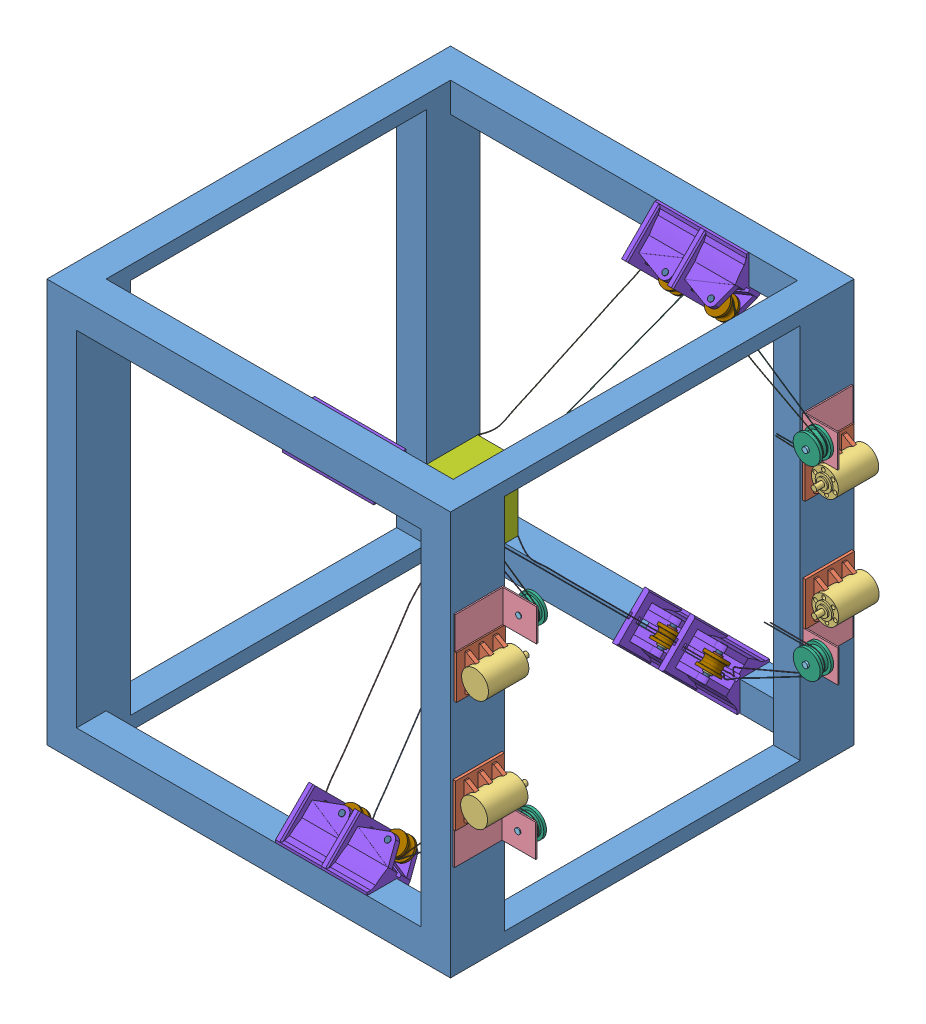
SolidWorks assembly 四自由度悬索机器人-粗装3, configuration 默认. Lengths in mm.
Overall size (1630.53 1500 1500).
86 component instances, 20 part files, 27 mates.
Components (placement in the parent):
- 框架-1: 框架 [默认] at (-869.4424 -713.1507 2250) size (1500 1500 1500)
- 驱动器-装配1-1: 驱动器-装配1 [默认] at (664.6049 -149.4407 667.2739) x (0 -1 0) z (0 0 1) size (280.09 130 239.56)
  - 驱动器--电机底座-1: 驱动器--电机底座 [默认] at (10.8985 -19.0474 121.978) size (160.09 50.28 181.98)
  - 驱动器-电机-1: 驱动器-电机 [默认] at (10.8985 30.9526 104.6663) x (0.931838 -0.362873 0) z (0 0 1) size (100 100 191)
  - 驱动器-滑轮组基座-1: 驱动器-滑轮组基座 [默认] at (90.9444 -34.0474 272.849) size (120 130 181.86)
  - 驱动器-定滑轮轴-1: 驱动器-定滑轮轴 [默认] at (150.9444 30.9526 265.5462) x (0.990128 -0.140168 0) z (0 0 1) size (20 20 65)
  - 驱动器-定滑轮-1: 驱动器-定滑轮 [默认] at (150.9167 30.9894 273.7821) x (0.990128 -0.140168 0) z (0 0 1) size (100 100 50)
- 驱动器-装配2-1: 驱动器-装配2 [默认] at (664.6049 262.8868 668.7376) x (0 -1 0) z (0 0 1) size (280.77 130.53 238.87)
  - 驱动器--电机底座-1: 驱动器--电机底座 [默认] at (10.8985 -19.0474 121.978) size (160.09 50.28 181.98)
  - 驱动器-电机-1: 驱动器-电机 [默认] at (10.8985 30.9526 104.6663) x (0.931838 -0.362873 0) z (0 0 1) size (100 100 191)
  - 驱动器-滑轮组基座-1: 驱动器-滑轮组基座 [默认] at (-189.8227 -33.5134 273.0905) size (120 130 181.86)
  - 驱动器-定滑轮轴-1: 驱动器-定滑轮轴 [默认] at (-129.7901 31.454 264.8545) size (20 20 65)
  - 驱动器-定滑轮-1: 驱动器-定滑轮 [默认] at (-129.8227 31.4866 273.0905) size (100 100 50)
- 驱动器-装配3-1: 驱动器-装配3 [默认] at (664.6049 -169.9542 2331.8379) x (0 1 0) z (0 0 -1) size (280.77 130.53 238.87)
  - 驱动器--电机底座-1: 驱动器--电机底座 [默认] at (10.8985 -19.0474 121.978) size (160.09 50.28 181.98)
  - 驱动器-电机-1: 驱动器-电机 [默认] at (10.8985 30.9526 104.6663) x (0.931838 -0.362873 0) z (0 0 1) size (100 100 191)
  - 驱动器-滑轮组基座-1: 驱动器-滑轮组基座 [默认] at (-189.8227 -33.5134 273.0905) size (120 130 181.86)
  - 驱动器-定滑轮轴-1: 驱动器-定滑轮轴 [默认] at (-129.7901 31.454 264.8545) size (20 20 65)
  - 驱动器-定滑轮-1: 驱动器-定滑轮 [默认] at (-129.8227 31.4866 273.0905) size (100 100 50)
- 驱动器-装配4-1: 驱动器-装配4 [默认] at (664.6049 241.4404 2328.4017) x (0 1 0) z (0 0 -1) size (280.09 130 239.56)
  - 驱动器--电机底座-1: 驱动器--电机底座 [默认] at (10.8985 -19.0474 121.978) size (160.09 50.28 181.98)
  - 驱动器-电机-1: 驱动器-电机 [默认] at (10.8985 30.9526 104.6663) x (0.931838 -0.362873 0) z (0 0 1) size (100 100 191)
  - 驱动器-滑轮组基座-1: 驱动器-滑轮组基座 [默认] at (90.9444 -34.0474 272.849) size (120 130 181.86)
  - 驱动器-定滑轮轴-1: 驱动器-定滑轮轴 [默认] at (150.9444 30.9526 265.5462) x (0.990128 -0.140168 0) z (0 0 1) size (20 20 65)
  - 驱动器-定滑轮-1: 驱动器-定滑轮 [默认] at (150.9167 30.9894 273.7821) x (0.990128 -0.140168 0) z (0 0 1) size (100 100 50)
- 执行器-1: 执行器 [默认] at (19.774 123.7995 1388.1997) x (0 -1 0) z (0 0 -1) size (250 150 200)
- 定滑轮组-装配1-2: 定滑轮组-装配1 [默认] at (151.3965 -782.1229 1166.7393) x (0 0 1) z (0 1 0) size (243.74 373.92 243.74)
  - 定滑轮-装配1-1: 定滑轮-装配1 [默认] at (-55.5304 53.8794 -79.4394) size (243.74 203.92 243.74)
    - 定滑轮-基座-1: 定滑轮-基座 [默认] at (-251.2089 -39.3736 258.4115) size (243.74 192.85 243.74)
    - 定滑轮-滚轮-1: 定滑轮-滚轮 [默认] at (-178.7162 65.1416 294.8732) x (0.51029 0.692249 0.51029) z (-0.707107 0 0.707107) size (80 80 50)
    - 定滑轮-轴-1: 定滑轮-轴 [默认] at (-153.8809 65.1416 270.0379) x (0.51029 0.692249 0.51029) z (-0.707107 0 0.707107) size (20 20 120)
    - 定滑轮-轴承1-1: 定滑轮-轴承1 [默认] at (-214.0716 65.1416 330.2286) x (0.51029 0.692249 0.51029) z (-0.707107 0 0.707107) size (30 30 5)
    - 定滑轮-轴承2-1: 定滑轮-轴承2 [默认] at (-175.1807 65.1416 291.3377) x (0.51029 0.692249 0.51029) z (-0.707107 0 0.707107) size (30 30 5)
  - 定滑轮-装配2-1: 定滑轮-装配2 [默认] at (-55.5304 -116.1206 -79.4394) size (243.74 203.92 243.74)
    - 定滑轮-基座-1: 定滑轮-基座 [默认] at (-251.2089 -39.3736 258.4115) size (243.74 192.85 243.74)
    - 定滑轮-滚轮-1: 定滑轮-滚轮 [默认] at (-178.7162 65.1416 294.8732) x (0.51029 0.692249 0.51029) z (-0.707107 0 0.707107) size (80 80 50)
    - 定滑轮-轴-1: 定滑轮-轴 [默认] at (-153.8809 65.1416 270.0379) x (0.51029 0.692249 0.51029) z (-0.707107 0 0.707107) size (20 20 120)
    - 定滑轮-轴承1-1: 定滑轮-轴承1 [默认] at (-214.0716 65.1416 330.2286) x (0.51029 0.692249 0.51029) z (-0.707107 0 0.707107) size (30 30 5)
    - 定滑轮-轴承2-1: 定滑轮-轴承2 [默认] at (-175.1807 65.1416 291.3377) x (0.51029 0.692249 0.51029) z (-0.707107 0 0.707107) size (30 30 5)
- 定滑轮组-装配2-1: 定滑轮组-装配2 [默认] at (155.9329 -296.4114 2318.9721) x (0 1 0) z (0 0 -1) size (243.74 373.92 243.74)
  - 定滑轮-装配1-1: 定滑轮-装配1 [默认] at (-55.5304 53.8794 -79.4394) size (243.74 203.92 243.74)
    - 定滑轮-基座-1: 定滑轮-基座 [默认] at (-251.2089 -39.3736 258.4115) size (243.74 192.85 243.74)
    - 定滑轮-滚轮-1: 定滑轮-滚轮 [默认] at (-178.7162 65.1416 294.8732) x (0.51029 0.692249 0.51029) z (-0.707107 0 0.707107) size (80 80 50)
    - 定滑轮-轴-1: 定滑轮-轴 [默认] at (-153.8809 65.1416 270.0379) x (0.51029 0.692249 0.51029) z (-0.707107 0 0.707107) size (20 20 120)
    - 定滑轮-轴承1-1: 定滑轮-轴承1 [默认] at (-214.0716 65.1416 330.2286) x (0.51029 0.692249 0.51029) z (-0.707107 0 0.707107) size (30 30 5)
    - 定滑轮-轴承2-1: 定滑轮-轴承2 [默认] at (-175.1807 65.1416 291.3377) x (0.51029 0.692249 0.51029) z (-0.707107 0 0.707107) size (30 30 5)
  - 定滑轮-装配2-1: 定滑轮-装配2 [默认] at (-55.5304 -116.1206 -79.4394) size (243.74 203.92 243.74)
    - 定滑轮-基座-1: 定滑轮-基座 [默认] at (-251.2089 -39.3736 258.4115) size (243.74 192.85 243.74)
    - 定滑轮-滚轮-1: 定滑轮-滚轮 [默认] at (-178.7162 65.1416 294.8732) x (0.51029 0.692249 0.51029) z (-0.707107 0 0.707107) size (80 80 50)
    - 定滑轮-轴-1: 定滑轮-轴 [默认] at (-153.8809 65.1416 270.0379) x (0.51029 0.692249 0.51029) z (-0.707107 0 0.707107) size (20 20 120)
    - 定滑轮-轴承1-1: 定滑轮-轴承1 [默认] at (-214.0716 65.1416 330.2286) x (0.51029 0.692249 0.51029) z (-0.707107 0 0.707107) size (30 30 5)
    - 定滑轮-轴承2-1: 定滑轮-轴承2 [默认] at (-175.1807 65.1416 291.3377) x (0.51029 0.692249 0.51029) z (-0.707107 0 0.707107) size (30 30 5)
- 定滑轮组-装配3-3: 定滑轮组-装配3 [默认] at (185.4984 370.1099 681.0279) x (0 -1 0) z (0 0 1) size (243.74 373.92 243.74)
  - 定滑轮-装配1-1: 定滑轮-装配1 [默认] at (-55.5304 53.8794 -79.4394) size (243.74 203.92 243.74)
    - 定滑轮-基座-1: 定滑轮-基座 [默认] at (-251.2089 -39.3736 258.4115) size (243.74 192.85 243.74)
    - 定滑轮-滚轮-1: 定滑轮-滚轮 [默认] at (-178.7162 65.1416 294.8732) x (0.51029 0.692249 0.51029) z (-0.707107 0 0.707107) size (80 80 50)
    - 定滑轮-轴-1: 定滑轮-轴 [默认] at (-153.8809 65.1416 270.0379) x (0.51029 0.692249 0.51029) z (-0.707107 0 0.707107) size (20 20 120)
    - 定滑轮-轴承1-1: 定滑轮-轴承1 [默认] at (-214.0716 65.1416 330.2286) x (0.51029 0.692249 0.51029) z (-0.707107 0 0.707107) size (30 30 5)
    - 定滑轮-轴承2-1: 定滑轮-轴承2 [默认] at (-175.1807 65.1416 291.3377) x (0.51029 0.692249 0.51029) z (-0.707107 0 0.707107) size (30 30 5)
  - 定滑轮-装配2-1: 定滑轮-装配2 [默认] at (-55.5304 -116.1206 -79.4394) size (243.74 203.92 243.74)
    - 定滑轮-基座-1: 定滑轮-基座 [默认] at (-251.2089 -39.3736 258.4115) size (243.74 192.85 243.74)
    - 定滑轮-滚轮-1: 定滑轮-滚轮 [默认] at (-178.7162 65.1416 294.8732) x (0.51029 0.692249 0.51029) z (-0.707107 0 0.707107) size (80 80 50)
    - 定滑轮-轴-1: 定滑轮-轴 [默认] at (-153.8809 65.1416 270.0379) x (0.51029 0.692249 0.51029) z (-0.707107 0 0.707107) size (20 20 120)
    - 定滑轮-轴承1-1: 定滑轮-轴承1 [默认] at (-214.0716 65.1416 330.2286) x (0.51029 0.692249 0.51029) z (-0.707107 0 0.707107) size (30 30 5)
    - 定滑轮-轴承2-1: 定滑轮-轴承2 [默认] at (-175.1807 65.1416 291.3377) x (0.51029 0.692249 0.51029) z (-0.707107 0 0.707107) size (30 30 5)
- 定滑轮组-装配4-2: 定滑轮组-装配4 [默认] at (180.9786 855.8214 1833.2607) x (0 0 -1) z (0 -1 0) size (243.74 373.92 243.74)
  - 定滑轮-装配1-1: 定滑轮-装配1 [默认] at (-55.5304 53.8794 -79.4394) size (243.74 203.92 243.74)
    - 定滑轮-基座-1: 定滑轮-基座 [默认] at (-251.2089 -39.3736 258.4115) size (243.74 192.85 243.74)
    - 定滑轮-滚轮-1: 定滑轮-滚轮 [默认] at (-178.7162 65.1416 294.8732) x (0.51029 0.692249 0.51029) z (-0.707107 0 0.707107) size (80 80 50)
    - 定滑轮-轴-1: 定滑轮-轴 [默认] at (-153.8809 65.1416 270.0379) x (0.51029 0.692249 0.51029) z (-0.707107 0 0.707107) size (20 20 120)
    - 定滑轮-轴承1-1: 定滑轮-轴承1 [默认] at (-214.0716 65.1416 330.2286) x (0.51029 0.692249 0.51029) z (-0.707107 0 0.707107) size (30 30 5)
    - 定滑轮-轴承2-1: 定滑轮-轴承2 [默认] at (-175.1807 65.1416 291.3377) x (0.51029 0.692249 0.51029) z (-0.707107 0 0.707107) size (30 30 5)
  - 定滑轮-装配2-1: 定滑轮-装配2 [默认] at (-55.5304 -116.1206 -79.4394) size (243.74 203.92 243.74)
    - 定滑轮-基座-1: 定滑轮-基座 [默认] at (-251.2089 -39.3736 258.4115) size (243.74 192.85 243.74)
    - 定滑轮-滚轮-1: 定滑轮-滚轮 [默认] at (-178.7162 65.1416 294.8732) x (0.51029 0.692249 0.51029) z (-0.707107 0 0.707107) size (80 80 50)
    - 定滑轮-轴-1: 定滑轮-轴 [默认] at (-153.8809 65.1416 270.0379) x (0.51029 0.692249 0.51029) z (-0.707107 0 0.707107) size (20 20 120)
    - 定滑轮-轴承1-1: 定滑轮-轴承1 [默认] at (-214.0716 65.1416 330.2286) x (0.51029 0.692249 0.51029) z (-0.707107 0 0.707107) size (30 30 5)
    - 定滑轮-轴承2-1: 定滑轮-轴承2 [默认] at (-175.1807 65.1416 291.3377) x (0.51029 0.692249 0.51029) z (-0.707107 0 0.707107) size (30 30 5)
- 绳1-1: 绳1 [默认] at origin size (718.73 546.46 497)
- 绳2-1: 绳2 [默认] at origin size (868.75 552.4 523.29)
- 绳3-1: 绳3 [默认] at origin size (723.76 427.02 492.19)
- 绳4-1: 绳4 [默认] at origin size (871.45 439.72 502.99)
- 绳5-1: 绳5 [默认] at origin size (743.88 445.89 515.69)
- 绳6-1: 绳6 [默认] at origin size (893.72 467.35 516.45)
- 绳7-1: 绳7 [默认] at origin size (721.1 554.76 527.15)
- 绳8-1: 绳8 [默认] at origin size (871.07 547.31 524.26)
Mates (geometry in assembly coordinates):
- 平行35: parallel: plane of assembly; plane of assembly; plane of 框架-1 through (520.5576 676.8493 2250) normal (-1 0 0); plane of 执行器-1 through (19.774 123.7995 1388.1997) normal (1 0 0)
- 平行36: parallel: plane of assembly; plane of assembly; plane of 框架-1 through (520.5576 676.8493 2250) normal (0 -1 0); plane of 执行器-1 through (-130.226 223.7995 1588.1997) normal (0 1 0)
- 平行37: parallel: plane of assembly; plane of assembly; plane of 框架-1 through (530.5576 786.8493 2140) normal (0 0 -1); plane of 执行器-1 through (-130.226 223.7995 1588.1997) normal (0 0 1)
- 平行38: parallel: plane of assembly; plane of assembly; plane of 框架-1 through (520.5576 676.8493 2250) normal (-1 0 0); plane of 定滑轮组-装配1-2/定滑轮-装配1-1/定滑轮-基座-1 through (315.9023 -603.1507 860) normal (1 0 0)
- 重合43: coincident: plane of assembly; plane of assembly; plane of 框架-1 through (530.5576 786.8493 860) normal (0 0 1); plane of 定滑轮组-装配1-2/定滑轮-装配1-1/定滑轮-基座-1 through (315.9023 -603.1507 860) normal (0 0 -1)
- 重合44: coincident: plane of assembly; plane of assembly; plane of 框架-1 through (520.5576 -603.1507 2250) normal (0 1 0); plane of 定滑轮组-装配1-2/定滑轮-装配1-1/定滑轮-基座-1 through (315.9023 -603.1507 750) normal (0 -1 0)
- 平行39: parallel: plane of 框架-1 through (520.5576 676.8493 2250) normal (-1 0 0); plane of 定滑轮组-装配2-1/定滑轮-装配1-1/定滑轮-基座-1 through (320.4388 -603.1507 2140) normal (1 0 0)
- 重合47: coincident: plane of 框架-1 through (520.5576 -603.1507 2250) normal (0 1 0); plane of 定滑轮组-装配2-1/定滑轮-装配1-1/定滑轮-基座-1 through (320.4388 -603.1507 2140) normal (0 -1 0)
- 重合48: coincident: plane of 框架-1 through (530.5576 786.8493 2140) normal (0 0 -1); plane of 定滑轮组-装配2-1/定滑轮-装配1-1/定滑轮-基座-1 through (320.4388 -713.1507 2140) normal (0 0 1)
- 平行41: parallel: plane of 框架-1 through (530.5576 786.8493 2140) normal (-1 0 0); plane of 定滑轮组-装配3-3/定滑轮-装配1-1/定滑轮-基座-1 through (350.0042 676.8493 860) normal (1 0 0)
- 重合52: coincident: plane of 框架-1 through (520.5576 676.8493 2250) normal (0 -1 0); plane of 定滑轮组-装配3-3/定滑轮-装配1-1/定滑轮-基座-1 through (350.0042 676.8493 860) normal (0 1 0)
- 重合53: coincident: plane of 框架-1 through (530.5576 786.8493 860) normal (0 0 1); plane of 定滑轮组-装配3-3/定滑轮-装配1-1/定滑轮-基座-1 through (350.0042 786.8493 860) normal (0 0 -1)
- 平行42: parallel: plane of 框架-1 through (520.5576 676.8493 2250) normal (-1 0 0); plane of 定滑轮组-装配4-2/定滑轮-装配1-1/定滑轮-基座-1 through (345.4844 676.8493 2140) normal (1 0 0)
- 重合55: coincident: plane of 框架-1 through (520.5576 676.8493 2250) normal (0 -1 0); plane of 定滑轮组-装配4-2/定滑轮-装配1-1/定滑轮-基座-1 through (345.4844 676.8493 2250) normal (0 1 0)
- 重合57: coincident: plane of 框架-1 through (530.5576 786.8493 2140) normal (0 0 -1); plane of 定滑轮组-装配4-2/定滑轮-装配1-1/定滑轮-基座-1 through (345.4844 676.8493 2140) normal (0 0 1)
- 重合62: coincident: plane of assembly; plane of assembly; plane of 框架-1 through (630.5576 786.8493 2250) normal (1 0 0); plane of 驱动器-装配1-1/驱动器--电机底座-1 through (630.5576 -160.3393 789.2519) normal (-1 0 0)
- 平行43: parallel: line of assembly; line of assembly; line of 框架-1 through (630.5576 786.8493 750) axis (0 -1 0); line of 驱动器-装配1-1/驱动器--电机底座-1 through (630.5576 -240.3851 758.2629) axis (0 1 0)
- 重合65: coincident: plane of 框架-1 through (630.5576 786.8493 2250) normal (1 0 0); plane of 驱动器-装配2-1/驱动器--电机底座-1 through (630.5576 251.9882 790.7156) normal (-1 0 0)
- 平行44: parallel: line of 框架-1 through (630.5576 786.8493 750) axis (0 -1 0); line of 驱动器-装配2-1/驱动器--电机底座-1 through (630.5576 171.9424 759.7266) axis (0 1 0)
- 重合68: coincident: plane of 框架-1 through (630.5576 786.8493 2250) normal (1 0 0); plane of 驱动器-装配3-1/驱动器--电机底座-1 through (630.5576 -159.0557 2209.8599) normal (-1 0 0)
- 平行45: parallel: line of 框架-1 through (630.5576 786.8493 2250) axis (0 -1 0); line of 驱动器-装配3-1/驱动器--电机底座-1 through (630.5576 -79.0098 2240.8489) axis (0 -1 0)
- 重合71: coincident: plane of assembly; plane of assembly; plane of 框架-1 through (630.5576 786.8493 2250) normal (1 0 0); plane of 驱动器-装配4-1/驱动器-滑轮组基座-1 through (630.5576 452.3848 2055.5527) normal (-1 0 0)
- 平行46: parallel: line of assembly; line of assembly; line of 框架-1 through (630.5576 786.8493 2250) axis (0 -1 0); line of 驱动器-装配4-1/驱动器-滑轮组基座-1 through (630.5576 452.3848 2237.4127) axis (0 -1 0)
- 重合74: coincident: point of 执行器-1; plane of ? through (19.774 -26.2005 1388.1997) normal (-0.400769 0.91152 0.092283)
- 重合75: coincident: unknown of 执行器-1; plane of ? through (19.7732 223.8004 1388.1998) normal (0.078521 -0.013988 0.996814)
- 重合77: coincident: unknown of 执行器-1; plane of ? through (19.774 -26.2005 1588.1997) normal (-0.808798 0.575683 0.120147)
- 重合78: coincident: unknown of 执行器-1; plane of ? through (-130.2235 223.7972 1588.1993) normal (0.287489 0.460465 -0.839835)
